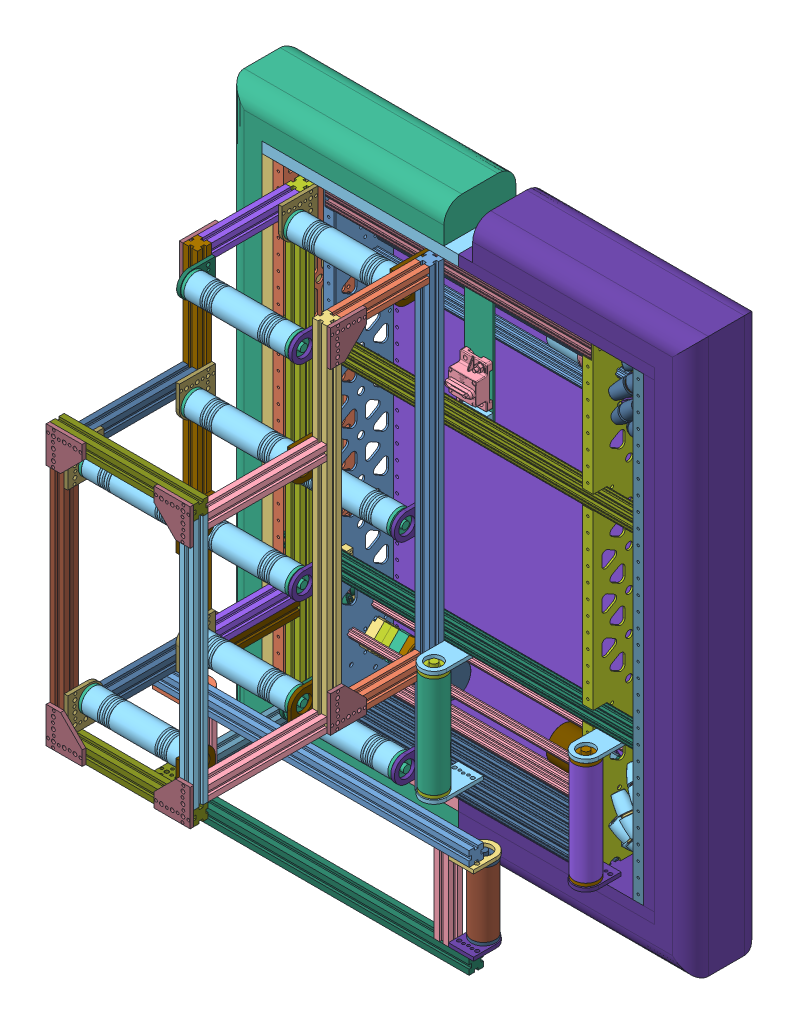
SolidWorks assembly Robot 2020, configuration Default. Lengths in mm. (continued)
Components (placement in the parent): (continued)
- Copy of Fame 2020-1: Copy of Fame 2020 [Default] at origin size (819.15 977.9 171.99) (continued)
  - NEO Gearbox 2-stage Custom v5(Mirror) (2)^Copy of Fame 2020-1: NEO Gearbox 2-stage Custom v5(Mirror) (2)^Copy of Fame 2020 [Default] at (0 0 425) x (1 0 0) z (0 0 -1) size (164.9 90.53 90.53) (virtual) (continued)
    - VersaPlanetary_4_1_Gear_Kit_217-2818 v1(Mirror) (2)^NEO Gearbox 2-stage Custom v5(Mirror) (2)_Copy of Fame 2020-1: VersaPlanetary_4_1_Gear_Kit_217-2818 v1(Mirror) (2)^NEO Gearbox 2-stage Custom v5(Mirror) (2)_Copy of Fame 2020 [Default] at (-15.25 22.225 0) x (0 -0.707107 -0.707107) z (1 0 0) size (35.49 35.49 17.4) (virtual) (continued)
      - 217-2625-010 Rev1(Mirror) (2)^VersaPlanetary_4_1_Gear_Kit_217-2818 v1(Mirror) (2)_NEO Gearbox 2-stage Custom v5(Mirror) (2)_Copy of Fame 2020-4: 217-2625-010 Rev1(Mirror) (2)^VersaPlanetary_4_1_Gear_Kit_217-2818 v1(Mirror) (2)_NEO Gearbox 2-stage Custom v5(Mirror) (2)_Copy of Fame 2020 [Default] at (-45.2382 -508.5855 214.725) x (0.519745 -0.854322 0) z (0 0 1) size (4 4 12) (virtual)
    - 217-2625-026 Rev1(Mirror) (2)^NEO Gearbox 2-stage Custom v5(Mirror) (2)_Copy of Fame 2020-1: 217-2625-026 Rev1(Mirror) (2)^NEO Gearbox 2-stage Custom v5(Mirror) (2)_Copy of Fame 2020 [Default] at (211.875 -317.5 391.6125) x (0 -0.707107 -0.707107) z (1 0 0) size (44.45 42 18.12) (virtual)
    - 217-2742-001 Rev4(Mirror) (2)^NEO Gearbox 2-stage Custom v5(Mirror) (2)_Copy of Fame 2020-1: 217-2742-001 Rev4(Mirror) (2)^NEO Gearbox 2-stage Custom v5(Mirror) (2)_Copy of Fame 2020 [Default] at (218.5752 -317.5 391.6125) x (1 0 0) z (0 -0.63857 0.769564) size (7 28 28) (virtual)
    - 217-2742-001 Rev4(Mirror) (2)^NEO Gearbox 2-stage Custom v5(Mirror) (2)_Copy of Fame 2020-2: 217-2742-001 Rev4(Mirror) (2)^NEO Gearbox 2-stage Custom v5(Mirror) (2)_Copy of Fame 2020 [Default] at (226.5752 -317.5 391.6125) x (1 0 0) z (0 -0.707107 0.707107) size (7 28 28) (virtual)
    - 217-2625-017 Rev1_9714K61(Mirror) (2)^NEO Gearbox 2-stage Custom v5(Mirror) (2)_Copy of Fame 2020-1: 217-2625-017 Rev1_9714K61(Mirror) (2)^NEO Gearbox 2-stage Custom v5(Mirror) (2)_Copy of Fame 2020 [Default] at (225.795 -317.6887 391.9075) x (0 0.983393 -0.181491) z (0 0.181491 0.983393) size (28.51 4.98 27.43) (virtual)
    - 217-2625-025 Rev1(Mirror) (2)^NEO Gearbox 2-stage Custom v5(Mirror) (2)_Copy of Fame 2020-1: 217-2625-025 Rev1(Mirror) (2)^NEO Gearbox 2-stage Custom v5(Mirror) (2)_Copy of Fame 2020 [Default] at (182.475 -317.5 391.6125) x (0 -0.707107 -0.707107) z (1 0 0) size (44.45 42 18) (virtual)
    - 217-2816-001 Rev1(Mirror) (2)^NEO Gearbox 2-stage Custom v5(Mirror) (2)_Copy of Fame 2020-1: 217-2816-001 Rev1(Mirror) (2)^NEO Gearbox 2-stage Custom v5(Mirror) (2)_Copy of Fame 2020 [Default] at (212.025 -317.5 391.6125) x (0 -0.707107 -0.707107) z (-1 0 0) size (42 42 14.5) (virtual)
    - 217-2816-001 Rev1(Mirror) (2)^NEO Gearbox 2-stage Custom v5(Mirror) (2)_Copy of Fame 2020-2: 217-2816-001 Rev1(Mirror) (2)^NEO Gearbox 2-stage Custom v5(Mirror) (2)_Copy of Fame 2020 [Default] at (199.325 -317.5 391.6125) x (0 -0.707107 -0.707107) z (-1 0 0) size (42 42 14.5) (virtual)
    - 217-4649-001 Rev1(Mirror) (2)^NEO Gearbox 2-stage Custom v5(Mirror) (2)_Copy of Fame 2020-1: 217-4649-001 Rev1(Mirror) (2)^NEO Gearbox 2-stage Custom v5(Mirror) (2)_Copy of Fame 2020 [Default] at (185.629 -317.5 391.6125) x (0 -0.707107 -0.707107) z (-1 0 0) size (18 18 13) (virtual)
    - VersaPlanetary_CIM_Adapter_217-4018 v1(Mirror) (2)^NEO Gearbox 2-stage Custom v5(Mirror) (2)_Copy of Fame 2020-1: VersaPlanetary_CIM_Adapter_217-4018 v1(Mirror) (2)^NEO Gearbox 2-stage Custom v5(Mirror) (2)_Copy of Fame 2020 [Default] at (165.15 -317.5 391.6125) x (0 -0.707107 -0.707107) z (0 -0.707107 0.707107) size (64.01 21.55 64.01) (virtual)
    - NEO Motor REV-21-1650 v2(Mirror) (2)^NEO Gearbox 2-stage Custom v5(Mirror) (2)_Copy of Fame 2020-1: NEO Motor REV-21-1650 v2(Mirror) (2)^NEO Gearbox 2-stage Custom v5(Mirror) (2)_Copy of Fame 2020 [Default] at (153.625 -317.5 391.6125) x (0 -0.707107 0.707107) z (-1 0 0) size (61.14 61.02 93.25) (virtual)
    - 3_1 Output Shaft Custom v6(Mirror) (2)^NEO Gearbox 2-stage Custom v5(Mirror) (2)_Copy of Fame 2020-1: 3_1 Output Shaft Custom v6(Mirror) (2)^NEO Gearbox 2-stage Custom v5(Mirror) (2)_Copy of Fame 2020 [Default] at (211.3752 -317.5 391.6125) x (1 0 0) z (0 -0.707107 0.707107) size (48.9 34.7 34.7) (virtual)
  - Left Wheel Assembly v4(Mirror) (2)^Copy of Fame 2020-1: Left Wheel Assembly v4(Mirror) (2)^Copy of Fame 2020 [Default] at (500 0 0) x (1 0 0) z (0 0 -1) size (65.82 166.11 165.01) (virtual)
    - 6_Mecanum_Wheel_Left_217-2799 v1(Mirror) (2)^Left Wheel Assembly v4(Mirror) (2)_Copy of Fame 2020-1: 6_Mecanum_Wheel_Left_217-2799 v1(Mirror) (2)^Left Wheel Assembly v4(Mirror) (2)_Copy of Fame 2020 [Default] x (0 0 -1) z (1 0 0) size (165.01 166.11 65.82) (virtual)
      - 217-2799-001 Rev1(Mirror) (2)^6_Mecanum_Wheel_Left_217-2799 v1(Mirror) (2)_Left Wheel Assembly v4(Mirror) (2)_Copy of Fame 2020-1: 217-2799-001 Rev1(Mirror) (2)^6_Mecanum_Wheel_Left_217-2799 v1(Mirror) (2)_Left Wheel Assembly v4(Mirror) (2)_Copy of Fame 2020 [Default] at (33.3875 -317.5 -234.0098) x (0.707107 0.707107 0) z (0 0 1) size (95.78 100.46 28.55) (virtual)
      - 217-2799-001 Rev1(Mirror) (2)^6_Mecanum_Wheel_Left_217-2799 v1(Mirror) (2)_Left Wheel Assembly v4(Mirror) (2)_Copy of Fame 2020-2: 217-2799-001 Rev1(Mirror) (2)^6_Mecanum_Wheel_Left_217-2799 v1(Mirror) (2)_Left Wheel Assembly v4(Mirror) (2)_Copy of Fame 2020 [Default] at (33.3875 -317.5 -221.3098) x (-0.987688 -0.156434 0) z (0 0 -1) size (95.78 100.46 28.55) (virtual)
      - 217-2799-002 Rev1(Mirror) (2)^6_Mecanum_Wheel_Left_217-2799 v1(Mirror) (2)_Left Wheel Assembly v4(Mirror) (2)_Copy of Fame 2020-1: 217-2799-002 Rev1(Mirror) (2)^6_Mecanum_Wheel_Left_217-2799 v1(Mirror) (2)_Left Wheel Assembly v4(Mirror) (2)_Copy of Fame 2020 [Default] at (4.057 -346.8305 -227.6598) x (-0.707107 0.707107 0) z (0.707107 0.707107 0) size (26.84 25.39 30.1) (virtual)
      - 217-2799-002 Rev1(Mirror) (2)^6_Mecanum_Wheel_Left_217-2799 v1(Mirror) (2)_Left Wheel Assembly v4(Mirror) (2)_Copy of Fame 2020-2: 217-2799-002 Rev1(Mirror) (2)^6_Mecanum_Wheel_Left_217-2799 v1(Mirror) (2)_Left Wheel Assembly v4(Mirror) (2)_Copy of Fame 2020 [Default] at (-7.5815 -323.9888 -227.6598) x (-0.156434 0.987688 0) z (0.987688 0.156434 0) size (26.84 25.39 30.1) (virtual)
      - 217-2799-002 Rev1(Mirror) (2)^6_Mecanum_Wheel_Left_217-2799 v1(Mirror) (2)_Left Wheel Assembly v4(Mirror) (2)_Copy of Fame 2020-3: 217-2799-002 Rev1(Mirror) (2)^6_Mecanum_Wheel_Left_217-2799 v1(Mirror) (2)_Left Wheel Assembly v4(Mirror) (2)_Copy of Fame 2020 [Default] at (-3.5711 -298.6686 -227.6598) x (0.45399 0.891007 0) z (0.891007 -0.45399 0) size (26.84 25.39 30.1) (virtual)
      - 217-2799-002 Rev1(Mirror) (2)^6_Mecanum_Wheel_Left_217-2799 v1(Mirror) (2)_Left Wheel Assembly v4(Mirror) (2)_Copy of Fame 2020-4: 217-2799-002 Rev1(Mirror) (2)^6_Mecanum_Wheel_Left_217-2799 v1(Mirror) (2)_Left Wheel Assembly v4(Mirror) (2)_Copy of Fame 2020 [Default] at (14.5561 -280.5414 -227.6598) x (0.891007 0.45399 0) z (0.45399 -0.891007 0) size (26.84 25.39 30.1) (virtual)
      - 217-2799-002 Rev1(Mirror) (2)^6_Mecanum_Wheel_Left_217-2799 v1(Mirror) (2)_Left Wheel Assembly v4(Mirror) (2)_Copy of Fame 2020-5: 217-2799-002 Rev1(Mirror) (2)^6_Mecanum_Wheel_Left_217-2799 v1(Mirror) (2)_Left Wheel Assembly v4(Mirror) (2)_Copy of Fame 2020 [Default] at (39.8763 -276.531 -227.6598) x (0.987688 -0.156434 0) z (-0.156434 -0.987688 0) size (26.84 25.39 30.1) (virtual)
      - 217-2799-002 Rev1(Mirror) (2)^6_Mecanum_Wheel_Left_217-2799 v1(Mirror) (2)_Left Wheel Assembly v4(Mirror) (2)_Copy of Fame 2020-6: 217-2799-002 Rev1(Mirror) (2)^6_Mecanum_Wheel_Left_217-2799 v1(Mirror) (2)_Left Wheel Assembly v4(Mirror) (2)_Copy of Fame 2020 [Default] at (62.718 -288.1695 -227.6598) x (0.707107 -0.707107 0) z (-0.707107 -0.707107 0) size (26.84 25.39 30.1) (virtual)
      - 217-2799-002 Rev1(Mirror) (2)^6_Mecanum_Wheel_Left_217-2799 v1(Mirror) (2)_Left Wheel Assembly v4(Mirror) (2)_Copy of Fame 2020-7: 217-2799-002 Rev1(Mirror) (2)^6_Mecanum_Wheel_Left_217-2799 v1(Mirror) (2)_Left Wheel Assembly v4(Mirror) (2)_Copy of Fame 2020 [Default] at (74.3565 -311.0112 -227.6598) x (0.156434 -0.987688 0) z (-0.987688 -0.156434 0) size (26.84 25.39 30.1) (virtual)
      - 217-2799-002 Rev1(Mirror) (2)^6_Mecanum_Wheel_Left_217-2799 v1(Mirror) (2)_Left Wheel Assembly v4(Mirror) (2)_Copy of Fame 2020-8: 217-2799-002 Rev1(Mirror) (2)^6_Mecanum_Wheel_Left_217-2799 v1(Mirror) (2)_Left Wheel Assembly v4(Mirror) (2)_Copy of Fame 2020 [Default] at (70.3461 -336.3314 -227.6598) x (-0.45399 -0.891007 0) z (-0.891007 0.45399 0) size (26.84 25.39 30.1) (virtual)
      - 217-2799-002 Rev1(Mirror) (2)^6_Mecanum_Wheel_Left_217-2799 v1(Mirror) (2)_Left Wheel Assembly v4(Mirror) (2)_Copy of Fame 2020-9: 217-2799-002 Rev1(Mirror) (2)^6_Mecanum_Wheel_Left_217-2799 v1(Mirror) (2)_Left Wheel Assembly v4(Mirror) (2)_Copy of Fame 2020 [Default] at (52.2189 -354.4586 -227.6598) x (-0.891007 -0.45399 0) z (-0.45399 0.891007 0) size (26.84 25.39 30.1) (virtual)
      - 217-2799-002 Rev1(Mirror) (2)^6_Mecanum_Wheel_Left_217-2799 v1(Mirror) (2)_Left Wheel Assembly v4(Mirror) (2)_Copy of Fame 2020-10: 217-2799-002 Rev1(Mirror) (2)^6_Mecanum_Wheel_Left_217-2799 v1(Mirror) (2)_Left Wheel Assembly v4(Mirror) (2)_Copy of Fame 2020 [Default] at (26.8987 -358.469 -227.6598) x (-0.987688 0.156434 0) z (0.156434 0.987688 0) size (26.84 25.39 30.1) (virtual)
      - 217-2586-003 Rev2(Mirror) (2)^6_Mecanum_Wheel_Left_217-2799 v1(Mirror) (2)_Left Wheel Assembly v4(Mirror) (2)_Copy of Fame 2020-1: 217-2586-003 Rev2(Mirror) (2)^6_Mecanum_Wheel_Left_217-2799 v1(Mirror) (2)_Left Wheel Assembly v4(Mirror) (2)_Copy of Fame 2020 [Default] at (-13.4676 -358.6894 -223.6536) x (0.41944 0.854155 -0.30739) z (0.757674 -0.142894 0.636798) size (19.46 28.57 19.46) (virtual)
      - 217-2586-003 Rev2(Mirror) (2)^6_Mecanum_Wheel_Left_217-2799 v1(Mirror) (2)_Left Wheel Assembly v4(Mirror) (2)_Copy of Fame 2020-2: 217-2586-003 Rev2(Mirror) (2)^6_Mecanum_Wheel_Left_217-2799 v1(Mirror) (2)_Left Wheel Assembly v4(Mirror) (2)_Copy of Fame 2020 [Default] at (-7.8019 -364.3551 -231.666) x (0.847342 0.451134 0.280161) z (-0.17892 0.739241 -0.649238) size (19.46 28.57 19.46) (virtual)
      - 217-2586-003 Rev2(Mirror) (2)^6_Mecanum_Wheel_Left_217-2799 v1(Mirror) (2)_Left Wheel Assembly v4(Mirror) (2)_Copy of Fame 2020-3: 217-2586-003 Rev2(Mirror) (2)^6_Mecanum_Wheel_Left_217-2799 v1(Mirror) (2)_Left Wheel Assembly v4(Mirror) (2)_Copy of Fame 2020 [Default] at (-27.4761 -331.196 -231.666) x (0.950684 -0.13308 0.280161) z (0.289766 0.703225 -0.649238) size (19.46 28.57 19.46) (virtual)
      - 217-2586-003 Rev2(Mirror) (2)^6_Mecanum_Wheel_Left_217-2799 v1(Mirror) (2)_Left Wheel Assembly v4(Mirror) (2)_Copy of Fame 2020-4: 217-2586-003 Rev2(Mirror) (2)^6_Mecanum_Wheel_Left_217-2799 v1(Mirror) (2)_Left Wheel Assembly v4(Mirror) (2)_Copy of Fame 2020 [Default] at (-23.9025 -292.8056 -231.666) x (0.690897 -0.666462 0.280161) z (0.647771 0.398601 -0.649238) size (19.46 28.57 19.46) (virtual)
      - 217-2586-003 Rev2(Mirror) (2)^6_Mecanum_Wheel_Left_217-2799 v1(Mirror) (2)_Left Wheel Assembly v4(Mirror) (2)_Copy of Fame 2020-5: 217-2586-003 Rev2(Mirror) (2)^6_Mecanum_Wheel_Left_217-2799 v1(Mirror) (2)_Left Wheel Assembly v4(Mirror) (2)_Copy of Fame 2020 [Default] at (1.5539 -263.8475 -231.666) x (0.167211 -0.945278 0.280161) z (0.75835 -0.058276 -0.649238) size (19.46 28.57 19.46) (virtual)
      - 217-2586-003 Rev2(Mirror) (2)^6_Mecanum_Wheel_Left_217-2799 v1(Mirror) (2)_Left Wheel Assembly v4(Mirror) (2)_Copy of Fame 2020-6: 217-2586-003 Rev2(Mirror) (2)^6_Mecanum_Wheel_Left_217-2799 v1(Mirror) (2)_Left Wheel Assembly v4(Mirror) (2)_Copy of Fame 2020 [Default] at (39.1697 -255.3829 -231.666) x (-0.420344 -0.86303 0.280161) z (0.579264 -0.492893 -0.649238) size (19.46 28.57 19.46) (virtual)
      - 217-2586-003 Rev2(Mirror) (2)^6_Mecanum_Wheel_Left_217-2799 v1(Mirror) (2)_Left Wheel Assembly v4(Mirror) (2)_Copy of Fame 2020-7: 217-2586-003 Rev2(Mirror) (2)^6_Mecanum_Wheel_Left_217-2799 v1(Mirror) (2)_Left Wheel Assembly v4(Mirror) (2)_Copy of Fame 2020 [Default] at (74.5769 -270.6449 -231.666) x (-0.847342 -0.451134 0.280161) z (0.17892 -0.739241 -0.649238) size (19.46 28.57 19.46) (virtual)
      - 217-2586-003 Rev2(Mirror) (2)^6_Mecanum_Wheel_Left_217-2799 v1(Mirror) (2)_Left Wheel Assembly v4(Mirror) (2)_Copy of Fame 2020-8: 217-2586-003 Rev2(Mirror) (2)^6_Mecanum_Wheel_Left_217-2799 v1(Mirror) (2)_Left Wheel Assembly v4(Mirror) (2)_Copy of Fame 2020 [Default] at (94.2511 -303.804 -231.666) x (-0.950684 0.13308 0.280161) z (-0.289766 -0.703225 -0.649238) size (19.46 28.57 19.46) (virtual)
      - 217-2586-003 Rev2(Mirror) (2)^6_Mecanum_Wheel_Left_217-2799 v1(Mirror) (2)_Left Wheel Assembly v4(Mirror) (2)_Copy of Fame 2020-9: 217-2586-003 Rev2(Mirror) (2)^6_Mecanum_Wheel_Left_217-2799 v1(Mirror) (2)_Left Wheel Assembly v4(Mirror) (2)_Copy of Fame 2020 [Default] at (90.6775 -342.1944 -231.666) x (-0.690897 0.666462 0.280161) z (-0.647771 -0.398601 -0.649238) size (19.46 28.57 19.46) (virtual)
      - 217-2586-003 Rev2(Mirror) (2)^6_Mecanum_Wheel_Left_217-2799 v1(Mirror) (2)_Left Wheel Assembly v4(Mirror) (2)_Copy of Fame 2020-10: 217-2586-003 Rev2(Mirror) (2)^6_Mecanum_Wheel_Left_217-2799 v1(Mirror) (2)_Left Wheel Assembly v4(Mirror) (2)_Copy of Fame 2020 [Default] at (65.2211 -371.1525 -231.666) x (-0.167211 0.945278 0.280161) z (-0.75835 0.058276 -0.649238) size (19.46 28.57 19.46) (virtual)
      - 217-2586-003 Rev2(Mirror) (2)^6_Mecanum_Wheel_Left_217-2799 v1(Mirror) (2)_Left Wheel Assembly v4(Mirror) (2)_Copy of Fame 2020-11: 217-2586-003 Rev2(Mirror) (2)^6_Mecanum_Wheel_Left_217-2799 v1(Mirror) (2)_Left Wheel Assembly v4(Mirror) (2)_Copy of Fame 2020 [Default] at (27.6053 -379.6171 -231.666) x (0.420344 0.86303 0.280161) z (-0.579264 0.492893 -0.649238) size (19.46 28.57 19.46) (virtual)
      - 217-2586-003 Rev2(Mirror) (2)^6_Mecanum_Wheel_Left_217-2799 v1(Mirror) (2)_Left Wheel Assembly v4(Mirror) (2)_Copy of Fame 2020-12: 217-2586-003 Rev2(Mirror) (2)^6_Mecanum_Wheel_Left_217-2799 v1(Mirror) (2)_Left Wheel Assembly v4(Mirror) (2)_Copy of Fame 2020 [Default] at (-28.7296 -323.2822 -223.6536) x (0.841394 0.444485 -0.30739) z (0.52898 -0.560953 0.636798) size (19.46 28.57 19.46) (virtual)
      - 217-2586-003 Rev2(Mirror) (2)^6_Mecanum_Wheel_Left_217-2799 v1(Mirror) (2)_Left Wheel Assembly v4(Mirror) (2)_Copy of Fame 2020-13: 217-2586-003 Rev2(Mirror) (2)^6_Mecanum_Wheel_Left_217-2799 v1(Mirror) (2)_Left Wheel Assembly v4(Mirror) (2)_Copy of Fame 2020 [Default] at (-20.265 -285.6664 -223.6536) x (0.941964 -0.134963 -0.30739) z (0.098234 -0.764747 0.636798) size (19.46 28.57 19.46) (virtual)
      - 217-2586-003 Rev2(Mirror) (2)^6_Mecanum_Wheel_Left_217-2799 v1(Mirror) (2)_Left Wheel Assembly v4(Mirror) (2)_Copy of Fame 2020-14: 217-2586-003 Rev2(Mirror) (2)^6_Mecanum_Wheel_Left_217-2799 v1(Mirror) (2)_Left Wheel Assembly v4(Mirror) (2)_Copy of Fame 2020 [Default] at (8.6931 -260.21 -223.6536) x (0.682736 -0.66286 -0.30739) z (-0.370035 -0.676434 0.636798) size (19.46 28.57 19.46) (virtual)
      - 217-2586-003 Rev2(Mirror) (2)^6_Mecanum_Wheel_Left_217-2799 v1(Mirror) (2)_Left Wheel Assembly v4(Mirror) (2)_Copy of Fame 2020-15: 217-2586-003 Rev2(Mirror) (2)^6_Mecanum_Wheel_Left_217-2799 v1(Mirror) (2)_Left Wheel Assembly v4(Mirror) (2)_Copy of Fame 2020 [Default] at (47.0835 -256.6364 -223.6536) x (0.162726 -0.937567 -0.30739) z (-0.696962 -0.329746 0.636798) size (19.46 28.57 19.46) (virtual)
      - 217-2586-003 Rev2(Mirror) (2)^6_Mecanum_Wheel_Left_217-2799 v1(Mirror) (2)_Left Wheel Assembly v4(Mirror) (2)_Copy of Fame 2020-16: 217-2586-003 Rev2(Mirror) (2)^6_Mecanum_Wheel_Left_217-2799 v1(Mirror) (2)_Left Wheel Assembly v4(Mirror) (2)_Copy of Fame 2020 [Default] at (80.2426 -276.3106 -223.6536) x (-0.41944 -0.854155 -0.30739) z (-0.757674 0.142894 0.636798) size (19.46 28.57 19.46) (virtual)
      - 217-2586-003 Rev2(Mirror) (2)^6_Mecanum_Wheel_Left_217-2799 v1(Mirror) (2)_Left Wheel Assembly v4(Mirror) (2)_Copy of Fame 2020-17: 217-2586-003 Rev2(Mirror) (2)^6_Mecanum_Wheel_Left_217-2799 v1(Mirror) (2)_Left Wheel Assembly v4(Mirror) (2)_Copy of Fame 2020 [Default] at (95.5046 -311.7178 -223.6536) x (-0.841394 -0.444485 -0.30739) z (-0.52898 0.560953 0.636798) size (19.46 28.57 19.46) (virtual)
      - 217-2586-003 Rev2(Mirror) (2)^6_Mecanum_Wheel_Left_217-2799 v1(Mirror) (2)_Left Wheel Assembly v4(Mirror) (2)_Copy of Fame 2020-18: 217-2586-003 Rev2(Mirror) (2)^6_Mecanum_Wheel_Left_217-2799 v1(Mirror) (2)_Left Wheel Assembly v4(Mirror) (2)_Copy of Fame 2020 [Default] at (87.04 -349.3336 -223.6536) x (-0.941964 0.134963 -0.30739) z (-0.098234 0.764747 0.636798) size (19.46 28.57 19.46) (virtual)
      - 217-2586-003 Rev2(Mirror) (2)^6_Mecanum_Wheel_Left_217-2799 v1(Mirror) (2)_Left Wheel Assembly v4(Mirror) (2)_Copy of Fame 2020-19: 217-2586-003 Rev2(Mirror) (2)^6_Mecanum_Wheel_Left_217-2799 v1(Mirror) (2)_Left Wheel Assembly v4(Mirror) (2)_Copy of Fame 2020 [Default] at (58.0819 -374.79 -223.6536) x (-0.682736 0.66286 -0.30739) z (0.370035 0.676434 0.636798) size (19.46 28.57 19.46) (virtual)
      - 217-2586-003 Rev2(Mirror) (2)^6_Mecanum_Wheel_Left_217-2799 v1(Mirror) (2)_Left Wheel Assembly v4(Mirror) (2)_Copy of Fame 2020-20: 217-2586-003 Rev2(Mirror) (2)^6_Mecanum_Wheel_Left_217-2799 v1(Mirror) (2)_Left Wheel Assembly v4(Mirror) (2)_Copy of Fame 2020 [Default] at (19.6915 -378.3636 -223.6536) x (-0.162726 0.937567 -0.30739) z (0.696962 0.329746 0.636798) size (19.46 28.57 19.46) (virtual)
      - 217-2586-004 Rev1(Mirror) (2)^6_Mecanum_Wheel_Left_217-2799 v1(Mirror) (2)_Left Wheel Assembly v4(Mirror) (2)_Copy of Fame 2020-1: 217-2586-004 Rev1(Mirror) (2)^6_Mecanum_Wheel_Left_217-2799 v1(Mirror) (2)_Left Wheel Assembly v4(Mirror) (2)_Copy of Fame 2020 [Default] at (-10.3479 -361.809 -228.0654) x (-0.690521 -0.722949 0.02293) z (-0.522667 0.476807 -0.706735) size (25.9 28.58 25.9) (virtual)
      - 217-2586-004 Rev1(Mirror) (2)^6_Mecanum_Wheel_Left_217-2799 v1(Mirror) (2)_Left Wheel Assembly v4(Mirror) (2)_Copy of Fame 2020-2: 217-2586-004 Rev1(Mirror) (2)^6_Mecanum_Wheel_Left_217-2799 v1(Mirror) (2)_Left Wheel Assembly v4(Mirror) (2)_Copy of Fame 2020 [Default] at (-10.9209 -361.2361 -227.2551) x (0.01458 -0.811521 0.584142) z (0.865903 0.302381 0.39847) size (25.9 28.58 25.9) (virtual)
      - 217-2586-004 Rev1(Mirror) (2)^6_Mecanum_Wheel_Left_217-2799 v1(Mirror) (2)_Left Wheel Assembly v4(Mirror) (2)_Copy of Fame 2020-3: 217-2586-004 Rev1(Mirror) (2)^6_Mecanum_Wheel_Left_217-2799 v1(Mirror) (2)_Left Wheel Assembly v4(Mirror) (2)_Copy of Fame 2020 [Default] at (-28.1662 -326.8394 -227.2551) x (-0.465204 -0.665104 0.584142) z (0.878265 -0.264334 0.39847) size (25.9 28.58 25.9) (virtual)
      - 217-2586-004 Rev1(Mirror) (2)^6_Mecanum_Wheel_Left_217-2799 v1(Mirror) (2)_Left Wheel Assembly v4(Mirror) (2)_Copy of Fame 2020-4: 217-2586-004 Rev1(Mirror) (2)^6_Mecanum_Wheel_Left_217-2799 v1(Mirror) (2)_Left Wheel Assembly v4(Mirror) (2)_Copy of Fame 2020 [Default] at (-21.9 -288.8754 -227.2551) x (-0.767297 -0.26464 0.584142) z (0.55516 -0.730082 0.39847) size (25.9 28.58 25.9) (virtual)
      - 217-2586-004 Rev1(Mirror) (2)^6_Mecanum_Wheel_Left_217-2799 v1(Mirror) (2)_Left Wheel Assembly v4(Mirror) (2)_Copy of Fame 2020-5: 217-2586-004 Rev1(Mirror) (2)^6_Mecanum_Wheel_Left_217-2799 v1(Mirror) (2)_Left Wheel Assembly v4(Mirror) (2)_Copy of Fame 2020 [Default] at (5.484 -261.845 -227.2551) x (-0.776308 0.236907 0.584142) z (0.020002 -0.916963 0.39847) size (25.9 28.58 25.9) (virtual)
      - 217-2586-004 Rev1(Mirror) (2)^6_Mecanum_Wheel_Left_217-2799 v1(Mirror) (2)_Left Wheel Assembly v4(Mirror) (2)_Copy of Fame 2020-6: 217-2586-004 Rev1(Mirror) (2)^6_Mecanum_Wheel_Left_217-2799 v1(Mirror) (2)_Left Wheel Assembly v4(Mirror) (2)_Copy of Fame 2020 [Default] at (43.5263 -256.0729 -227.2551) x (-0.488796 0.647964 0.584142) z (-0.522795 -0.753596 0.39847) size (25.9 28.58 25.9) (virtual)
      - 217-2586-004 Rev1(Mirror) (2)^6_Mecanum_Wheel_Left_217-2799 v1(Mirror) (2)_Left Wheel Assembly v4(Mirror) (2)_Copy of Fame 2020-7: 217-2586-004 Rev1(Mirror) (2)^6_Mecanum_Wheel_Left_217-2799 v1(Mirror) (2)_Left Wheel Assembly v4(Mirror) (2)_Copy of Fame 2020 [Default] at (77.6959 -273.7639 -227.2551) x (-0.01458 0.811521 0.584142) z (-0.865903 -0.302381 0.39847) size (25.9 28.58 25.9) (virtual)
      - 217-2586-004 Rev1(Mirror) (2)^6_Mecanum_Wheel_Left_217-2799 v1(Mirror) (2)_Left Wheel Assembly v4(Mirror) (2)_Copy of Fame 2020-8: 217-2586-004 Rev1(Mirror) (2)^6_Mecanum_Wheel_Left_217-2799 v1(Mirror) (2)_Left Wheel Assembly v4(Mirror) (2)_Copy of Fame 2020 [Default] at (94.9412 -308.1606 -227.2551) x (0.465204 0.665104 0.584142) z (-0.878265 0.264334 0.39847) size (25.9 28.58 25.9) (virtual)
      - 217-2586-004 Rev1(Mirror) (2)^6_Mecanum_Wheel_Left_217-2799 v1(Mirror) (2)_Left Wheel Assembly v4(Mirror) (2)_Copy of Fame 2020-9: 217-2586-004 Rev1(Mirror) (2)^6_Mecanum_Wheel_Left_217-2799 v1(Mirror) (2)_Left Wheel Assembly v4(Mirror) (2)_Copy of Fame 2020 [Default] at (88.675 -346.1246 -227.2551) x (0.767297 0.26464 0.584142) z (-0.55516 0.730082 0.39847) size (25.9 28.58 25.9) (virtual)
      - 217-2586-004 Rev1(Mirror) (2)^6_Mecanum_Wheel_Left_217-2799 v1(Mirror) (2)_Left Wheel Assembly v4(Mirror) (2)_Copy of Fame 2020-10: 217-2586-004 Rev1(Mirror) (2)^6_Mecanum_Wheel_Left_217-2799 v1(Mirror) (2)_Left Wheel Assembly v4(Mirror) (2)_Copy of Fame 2020 [Default] at (61.291 -373.155 -227.2551) x (0.776308 -0.236907 0.584142) z (-0.020002 0.916963 0.39847) size (25.9 28.58 25.9) (virtual)
      - 217-2586-004 Rev1(Mirror) (2)^6_Mecanum_Wheel_Left_217-2799 v1(Mirror) (2)_Left Wheel Assembly v4(Mirror) (2)_Copy of Fame 2020-11: 217-2586-004 Rev1(Mirror) (2)^6_Mecanum_Wheel_Left_217-2799 v1(Mirror) (2)_Left Wheel Assembly v4(Mirror) (2)_Copy of Fame 2020 [Default] at (23.2487 -378.9271 -227.2551) x (0.488796 -0.647964 0.584142) z (0.522795 0.753596 0.39847) size (25.9 28.58 25.9) (virtual)
      - 217-2586-004 Rev1(Mirror) (2)^6_Mecanum_Wheel_Left_217-2799 v1(Mirror) (2)_Left Wheel Assembly v4(Mirror) (2)_Copy of Fame 2020-12: 217-2586-004 Rev1(Mirror) (2)^6_Mecanum_Wheel_Left_217-2799 v1(Mirror) (2)_Left Wheel Assembly v4(Mirror) (2)_Copy of Fame 2020 [Default] at (-28.0394 -327.6397 -228.0654) x (-0.983582 -0.179 0.02293) z (-0.142587 0.692961 -0.706735) size (25.9 28.58 25.9) (virtual)
      - 217-2586-004 Rev1(Mirror) (2)^6_Mecanum_Wheel_Left_217-2799 v1(Mirror) (2)_Left Wheel Assembly v4(Mirror) (2)_Copy of Fame 2020-13: 217-2586-004 Rev1(Mirror) (2)^6_Mecanum_Wheel_Left_217-2799 v1(Mirror) (2)_Left Wheel Assembly v4(Mirror) (2)_Copy of Fame 2020 [Default] at (-22.2679 -289.5974 -228.0654) x (-0.900948 0.433321 0.02293) z (0.291957 0.644427 -0.706735) size (25.9 28.58 25.9) (virtual)
      - 217-2586-004 Rev1(Mirror) (2)^6_Mecanum_Wheel_Left_217-2799 v1(Mirror) (2)_Left Wheel Assembly v4(Mirror) (2)_Copy of Fame 2020-14: 217-2586-004 Rev1(Mirror) (2)^6_Mecanum_Wheel_Left_217-2799 v1(Mirror) (2)_Left Wheel Assembly v4(Mirror) (2)_Copy of Fame 2020 [Default] at (4.7621 -262.2129 -228.0654) x (-0.474183 0.880128 0.02293) z (0.614983 0.349745 -0.706735) size (25.9 28.58 25.9) (virtual)
      - 217-2586-004 Rev1(Mirror) (2)^6_Mecanum_Wheel_Left_217-2799 v1(Mirror) (2)_Left Wheel Assembly v4(Mirror) (2)_Copy of Fame 2020-15: 217-2586-004 Rev1(Mirror) (2)^6_Mecanum_Wheel_Left_217-2799 v1(Mirror) (2)_Left Wheel Assembly v4(Mirror) (2)_Copy of Fame 2020 [Default] at (42.726 -255.9462 -228.0654) x (0.133704 0.990756 0.02293) z (0.703107 -0.078529 -0.706735) size (25.9 28.58 25.9) (virtual)
      - 217-2586-004 Rev1(Mirror) (2)^6_Mecanum_Wheel_Left_217-2799 v1(Mirror) (2)_Left Wheel Assembly v4(Mirror) (2)_Copy of Fame 2020-16: 217-2586-004 Rev1(Mirror) (2)^6_Mecanum_Wheel_Left_217-2799 v1(Mirror) (2)_Left Wheel Assembly v4(Mirror) (2)_Copy of Fame 2020 [Default] at (77.1229 -273.191 -228.0654) x (0.690521 0.722949 0.02293) z (0.522667 -0.476807 -0.706735) size (25.9 28.58 25.9) (virtual)
      - 217-2586-004 Rev1(Mirror) (2)^6_Mecanum_Wheel_Left_217-2799 v1(Mirror) (2)_Left Wheel Assembly v4(Mirror) (2)_Copy of Fame 2020-17: 217-2586-004 Rev1(Mirror) (2)^6_Mecanum_Wheel_Left_217-2799 v1(Mirror) (2)_Left Wheel Assembly v4(Mirror) (2)_Copy of Fame 2020 [Default] at (94.8144 -307.3603 -228.0654) x (0.983582 0.179 0.02293) z (0.142587 -0.692961 -0.706735) size (25.9 28.58 25.9) (virtual)
      - 217-2586-004 Rev1(Mirror) (2)^6_Mecanum_Wheel_Left_217-2799 v1(Mirror) (2)_Left Wheel Assembly v4(Mirror) (2)_Copy of Fame 2020-18: 217-2586-004 Rev1(Mirror) (2)^6_Mecanum_Wheel_Left_217-2799 v1(Mirror) (2)_Left Wheel Assembly v4(Mirror) (2)_Copy of Fame 2020 [Default] at (89.0429 -345.4026 -228.0654) x (0.900948 -0.433321 0.02293) z (-0.291957 -0.644427 -0.706735) size (25.9 28.58 25.9) (virtual)
      - 217-2586-004 Rev1(Mirror) (2)^6_Mecanum_Wheel_Left_217-2799 v1(Mirror) (2)_Left Wheel Assembly v4(Mirror) (2)_Copy of Fame 2020-19: 217-2586-004 Rev1(Mirror) (2)^6_Mecanum_Wheel_Left_217-2799 v1(Mirror) (2)_Left Wheel Assembly v4(Mirror) (2)_Copy of Fame 2020 [Default] at (62.0129 -372.7871 -228.0654) x (0.474183 -0.880128 0.02293) z (-0.614983 -0.349745 -0.706735) size (25.9 28.58 25.9) (virtual)
      - 217-2586-004 Rev1(Mirror) (2)^6_Mecanum_Wheel_Left_217-2799 v1(Mirror) (2)_Left Wheel Assembly v4(Mirror) (2)_Copy of Fame 2020-20: 217-2586-004 Rev1(Mirror) (2)^6_Mecanum_Wheel_Left_217-2799 v1(Mirror) (2)_Left Wheel Assembly v4(Mirror) (2)_Copy of Fame 2020 [Default] at (24.049 -379.0538 -228.0654) x (-0.133704 -0.990756 0.02293) z (-0.703107 0.078529 -0.706735) size (25.9 28.58 25.9) (virtual)
      - 217-2586-007 Rev1(Mirror) (2)^6_Mecanum_Wheel_Left_217-2799 v1(Mirror) (2)_Left Wheel Assembly v4(Mirror) (2)_Copy of Fame 2020-1: 217-2586-007 Rev1(Mirror) (2)^6_Mecanum_Wheel_Left_217-2799 v1(Mirror) (2)_Left Wheel Assembly v4(Mirror) (2)_Copy of Fame 2020 [Default] at (-10.6347 -361.5222 -227.6598) x (0.5 -0.5 -0.707107) z (0.709055 0.705148 0.002763) size (61.72 5 5) (virtual)
      - 217-2586-007 Rev1(Mirror) (2)^6_Mecanum_Wheel_Left_217-2799 v1(Mirror) (2)_Left Wheel Assembly v4(Mirror) (2)_Copy of Fame 2020-2: 217-2586-007 Rev1(Mirror) (2)^6_Mecanum_Wheel_Left_217-2799 v1(Mirror) (2)_Left Wheel Assembly v4(Mirror) (2)_Copy of Fame 2020 [Default] at (-28.1029 -327.2391 -227.6598) x (0.110616 -0.698401 -0.707107) z (0.988113 0.153705 0.002763) size (61.72 5 5) (virtual)
      - 217-2586-007 Rev1(Mirror) (2)^6_Mecanum_Wheel_Left_217-2799 v1(Mirror) (2)_Left Wheel Assembly v4(Mirror) (2)_Copy of Fame 2020-3: 217-2586-007 Rev1(Mirror) (2)^6_Mecanum_Wheel_Left_217-2799 v1(Mirror) (2)_Left Wheel Assembly v4(Mirror) (2)_Copy of Fame 2020 [Default] at (-22.0838 -289.236 -227.6598) x (-0.32102 -0.630037 -0.707107) z (0.889746 -0.456448 0.002763) size (61.72 5 5) (virtual)
      - 217-2586-007 Rev1(Mirror) (2)^6_Mecanum_Wheel_Left_217-2799 v1(Mirror) (2)_Left Wheel Assembly v4(Mirror) (2)_Copy of Fame 2020-4: 217-2586-007 Rev1(Mirror) (2)^6_Mecanum_Wheel_Left_217-2799 v1(Mirror) (2)_Left Wheel Assembly v4(Mirror) (2)_Copy of Fame 2020 [Default] at (5.1235 -262.0287 -227.6598) x (-0.630037 -0.32102 -0.707107) z (0.451526 -0.892254 0.002763) size (61.72 5 5) (virtual)
      - 217-2586-007 Rev1(Mirror) (2)^6_Mecanum_Wheel_Left_217-2799 v1(Mirror) (2)_Left Wheel Assembly v4(Mirror) (2)_Copy of Fame 2020-5: 217-2586-007 Rev1(Mirror) (2)^6_Mecanum_Wheel_Left_217-2799 v1(Mirror) (2)_Left Wheel Assembly v4(Mirror) (2)_Copy of Fame 2020 [Default] at (43.1266 -256.0096 -227.6598) x (-0.698401 0.110616 -0.707107) z (-0.159162 -0.987249 0.002763) size (61.72 5 5) (virtual)
      - 217-2586-007 Rev1(Mirror) (2)^6_Mecanum_Wheel_Left_217-2799 v1(Mirror) (2)_Left Wheel Assembly v4(Mirror) (2)_Copy of Fame 2020-6: 217-2586-007 Rev1(Mirror) (2)^6_Mecanum_Wheel_Left_217-2799 v1(Mirror) (2)_Left Wheel Assembly v4(Mirror) (2)_Copy of Fame 2020 [Default] at (77.4097 -273.4778 -227.6598) x (-0.5 0.5 -0.707107) z (-0.709055 -0.705148 0.002763) size (61.72 5 5) (virtual)
      - 217-2586-007 Rev1(Mirror) (2)^6_Mecanum_Wheel_Left_217-2799 v1(Mirror) (2)_Left Wheel Assembly v4(Mirror) (2)_Copy of Fame 2020-7: 217-2586-007 Rev1(Mirror) (2)^6_Mecanum_Wheel_Left_217-2799 v1(Mirror) (2)_Left Wheel Assembly v4(Mirror) (2)_Copy of Fame 2020 [Default] at (94.8779 -307.7609 -227.6598) x (-0.110616 0.698401 -0.707107) z (-0.988113 -0.153705 0.002763) size (61.72 5 5) (virtual)
      - 217-2586-007 Rev1(Mirror) (2)^6_Mecanum_Wheel_Left_217-2799 v1(Mirror) (2)_Left Wheel Assembly v4(Mirror) (2)_Copy of Fame 2020-8: 217-2586-007 Rev1(Mirror) (2)^6_Mecanum_Wheel_Left_217-2799 v1(Mirror) (2)_Left Wheel Assembly v4(Mirror) (2)_Copy of Fame 2020 [Default] at (88.8588 -345.764 -227.6598) x (0.32102 0.630037 -0.707107) z (-0.889746 0.456448 0.002763) size (61.72 5 5) (virtual)
      - 217-2586-007 Rev1(Mirror) (2)^6_Mecanum_Wheel_Left_217-2799 v1(Mirror) (2)_Left Wheel Assembly v4(Mirror) (2)_Copy of Fame 2020-9: 217-2586-007 Rev1(Mirror) (2)^6_Mecanum_Wheel_Left_217-2799 v1(Mirror) (2)_Left Wheel Assembly v4(Mirror) (2)_Copy of Fame 2020 [Default] at (61.6515 -372.9713 -227.6598) x (0.630037 0.32102 -0.707107) z (-0.451526 0.892254 0.002763) size (61.72 5 5) (virtual)
      - 217-2586-007 Rev1(Mirror) (2)^6_Mecanum_Wheel_Left_217-2799 v1(Mirror) (2)_Left Wheel Assembly v4(Mirror) (2)_Copy of Fame 2020-10: 217-2586-007 Rev1(Mirror) (2)^6_Mecanum_Wheel_Left_217-2799 v1(Mirror) (2)_Left Wheel Assembly v4(Mirror) (2)_Copy of Fame 2020 [Default] at (23.6484 -378.9904 -227.6598) x (0.698401 -0.110616 -0.707107) z (0.159162 0.987249 0.002763) size (61.72 5 5) (virtual)
      - 217-2586-008 Rev1(Mirror) (2)^6_Mecanum_Wheel_Left_217-2799 v1(Mirror) (2)_Left Wheel Assembly v4(Mirror) (2)_Copy of Fame 2020-1: 217-2586-008 Rev1(Mirror) (2)^6_Mecanum_Wheel_Left_217-2799 v1(Mirror) (2)_Left Wheel Assembly v4(Mirror) (2)_Copy of Fame 2020 [Default] at (53.3583 -330.4692 -227.5328) x (0.544639 0.838671 0) z (0 0 -1) size (7.33 6.35 31.75) (virtual)
      - 217-2586-008 Rev1(Mirror) (2)^6_Mecanum_Wheel_Left_217-2799 v1(Mirror) (2)_Left Wheel Assembly v4(Mirror) (2)_Copy of Fame 2020-2: 217-2586-008 Rev1(Mirror) (2)^6_Mecanum_Wheel_Left_217-2799 v1(Mirror) (2)_Left Wheel Assembly v4(Mirror) (2)_Copy of Fame 2020 [Default] at (32.1413 -341.2799 -227.5328) x (0.99863 -0.052336 0) z (0 0 -1) size (7.33 6.35 31.75) (virtual)
      - 217-2586-008 Rev1(Mirror) (2)^6_Mecanum_Wheel_Left_217-2799 v1(Mirror) (2)_Left Wheel Assembly v4(Mirror) (2)_Copy of Fame 2020-3: 217-2586-008 Rev1(Mirror) (2)^6_Mecanum_Wheel_Left_217-2799 v1(Mirror) (2)_Left Wheel Assembly v4(Mirror) (2)_Copy of Fame 2020 [Default] at (12.1704 -328.3106 -227.5328) x (0.45399 -0.891007 0) z (0 0 -1) size (7.33 6.35 31.75) (virtual)
      - 217-2586-008 Rev1(Mirror) (2)^6_Mecanum_Wheel_Left_217-2799 v1(Mirror) (2)_Left Wheel Assembly v4(Mirror) (2)_Copy of Fame 2020-4: 217-2586-008 Rev1(Mirror) (2)^6_Mecanum_Wheel_Left_217-2799 v1(Mirror) (2)_Left Wheel Assembly v4(Mirror) (2)_Copy of Fame 2020 [Default] at (13.4167 -304.5308 -227.5328) x (-0.544639 -0.838671 0) z (0 0 -1) size (7.33 6.35 31.75) (virtual)
      - 217-2586-008 Rev1(Mirror) (2)^6_Mecanum_Wheel_Left_217-2799 v1(Mirror) (2)_Left Wheel Assembly v4(Mirror) (2)_Copy of Fame 2020-5: 217-2586-008 Rev1(Mirror) (2)^6_Mecanum_Wheel_Left_217-2799 v1(Mirror) (2)_Left Wheel Assembly v4(Mirror) (2)_Copy of Fame 2020 [Default] at (34.6337 -293.7201 -227.5328) x (-0.99863 0.052336 0) z (0 0 -1) size (7.33 6.35 31.75) (virtual)
      - 217-2586-008 Rev1(Mirror) (2)^6_Mecanum_Wheel_Left_217-2799 v1(Mirror) (2)_Left Wheel Assembly v4(Mirror) (2)_Copy of Fame 2020-6: 217-2586-008 Rev1(Mirror) (2)^6_Mecanum_Wheel_Left_217-2799 v1(Mirror) (2)_Left Wheel Assembly v4(Mirror) (2)_Copy of Fame 2020 [Default] at (54.6046 -306.6894 -227.5328) x (-0.45399 0.891007 0) z (0 0 -1) size (7.33 6.35 31.75) (virtual)
      - NUT-832-NYLOCK(Mirror) (2)^6_Mecanum_Wheel_Left_217-2799 v1(Mirror) (2)_Left Wheel Assembly v4(Mirror) (2)_Copy of Fame 2020-1: NUT-832-NYLOCK(Mirror) (2)^6_Mecanum_Wheel_Left_217-2799 v1(Mirror) (2)_Left Wheel Assembly v4(Mirror) (2)_Copy of Fame 2020 [Default] at (6.1639 -290.2764 -241.3161) x (0.258819 -0.965926 0) z (0.965926 0.258819 0) size (9.37 5.86 8.12) (virtual)
      - NUT-832-NYLOCK(Mirror) (2)^6_Mecanum_Wheel_Left_217-2799 v1(Mirror) (2)_Left Wheel Assembly v4(Mirror) (2)_Copy of Fame 2020-2: NUT-832-NYLOCK(Mirror) (2)^6_Mecanum_Wheel_Left_217-2799 v1(Mirror) (2)_Left Wheel Assembly v4(Mirror) (2)_Copy of Fame 2020 [Default] at (-0.9163 -334.9786 -241.3161) x (0.99863 -0.052336 0) z (0.052336 0.99863 0) size (9.37 5.86 8.12) (virtual)
      - NUT-832-NYLOCK(Mirror) (2)^6_Mecanum_Wheel_Left_217-2799 v1(Mirror) (2)_Left Wheel Assembly v4(Mirror) (2)_Copy of Fame 2020-3: NUT-832-NYLOCK(Mirror) (2)^6_Mecanum_Wheel_Left_217-2799 v1(Mirror) (2)_Left Wheel Assembly v4(Mirror) (2)_Copy of Fame 2020 [Default] at (39.4102 -355.526 -241.3161) x (0.358368 0.93358 0) z (-0.93358 0.358368 0) size (9.37 5.86 8.12) (virtual)
      - NUT-832-NYLOCK(Mirror) (2)^6_Mecanum_Wheel_Left_217-2799 v1(Mirror) (2)_Left Wheel Assembly v4(Mirror) (2)_Copy of Fame 2020-4: NUT-832-NYLOCK(Mirror) (2)^6_Mecanum_Wheel_Left_217-2799 v1(Mirror) (2)_Left Wheel Assembly v4(Mirror) (2)_Copy of Fame 2020 [Default] at (71.4135 -323.5227 -241.3161) x (-0.777146 0.62932 0) z (-0.62932 -0.777146 0) size (9.37 5.86 8.12) (virtual)
      - NUT-832-NYLOCK(Mirror) (2)^6_Mecanum_Wheel_Left_217-2799 v1(Mirror) (2)_Left Wheel Assembly v4(Mirror) (2)_Copy of Fame 2020-5: NUT-832-NYLOCK(Mirror) (2)^6_Mecanum_Wheel_Left_217-2799 v1(Mirror) (2)_Left Wheel Assembly v4(Mirror) (2)_Copy of Fame 2020 [Default] at (50.8661 -283.1962 -241.3161) x (-0.838671 -0.544639 0) z (0.544639 -0.838671 0) size (9.37 5.86 8.12) (virtual)
      - SCREW-832-1250(Mirror) (2)^6_Mecanum_Wheel_Left_217-2799 v1(Mirror) (2)_Left Wheel Assembly v4(Mirror) (2)_Copy of Fame 2020-1: SCREW-832-1250(Mirror) (2)^6_Mecanum_Wheel_Left_217-2799 v1(Mirror) (2)_Left Wheel Assembly v4(Mirror) (2)_Copy of Fame 2020 [Default] at (6.1639 -290.2764 -212.75) x (0 0 -1) z (0.394243 -0.919006 0) size (33.96 7.92 7.92) (virtual)
      - SCREW-832-1250(Mirror) (2)^6_Mecanum_Wheel_Left_217-2799 v1(Mirror) (2)_Left Wheel Assembly v4(Mirror) (2)_Copy of Fame 2020-2: SCREW-832-1250(Mirror) (2)^6_Mecanum_Wheel_Left_217-2799 v1(Mirror) (2)_Left Wheel Assembly v4(Mirror) (2)_Copy of Fame 2020 [Default] at (-0.9163 -334.9786 -212.75) x (0 0 -1) z (0.995855 0.090959 0) size (33.96 7.92 7.92) (virtual)
      - SCREW-832-1250(Mirror) (2)^6_Mecanum_Wheel_Left_217-2799 v1(Mirror) (2)_Left Wheel Assembly v4(Mirror) (2)_Copy of Fame 2020-3: SCREW-832-1250(Mirror) (2)^6_Mecanum_Wheel_Left_217-2799 v1(Mirror) (2)_Left Wheel Assembly v4(Mirror) (2)_Copy of Fame 2020 [Default] at (39.4102 -355.526 -212.75) x (0 0 -1) z (0.221229 0.975222 0) size (33.96 7.92 7.92) (virtual)
      - SCREW-832-1250(Mirror) (2)^6_Mecanum_Wheel_Left_217-2799 v1(Mirror) (2)_Left Wheel Assembly v4(Mirror) (2)_Copy of Fame 2020-4: SCREW-832-1250(Mirror) (2)^6_Mecanum_Wheel_Left_217-2799 v1(Mirror) (2)_Left Wheel Assembly v4(Mirror) (2)_Copy of Fame 2020 [Default] at (71.4135 -323.5227 -212.75) x (0 0 -1) z (-0.859128 0.511761 0) size (33.96 7.92 7.92) (virtual)
      - SCREW-832-1250(Mirror) (2)^6_Mecanum_Wheel_Left_217-2799 v1(Mirror) (2)_Left Wheel Assembly v4(Mirror) (2)_Copy of Fame 2020-5: SCREW-832-1250(Mirror) (2)^6_Mecanum_Wheel_Left_217-2799 v1(Mirror) (2)_Left Wheel Assembly v4(Mirror) (2)_Copy of Fame 2020 [Default] at (50.8661 -283.1962 -212.75) x (0 0 -1) z (-0.752199 -0.658936 0) size (33.96 7.92 7.92) (virtual)
      - 217-2586-005 Rev2(Mirror) (2)^6_Mecanum_Wheel_Left_217-2799 v1(Mirror) (2)_Left Wheel Assembly v4(Mirror) (2)_Copy of Fame 2020-1: 217-2586-005 Rev2(Mirror) (2)^6_Mecanum_Wheel_Left_217-2799 v1(Mirror) (2)_Left Wheel Assembly v4(Mirror) (2)_Copy of Fame 2020 [Default] at (-6.1597 -365.9972 -233.9884) x (-0.5 0.5 0.707107) z (-0.146447 -0.853553 0.5) size (8.5 8 8) (virtual)
      - 217-2586-005 Rev2(Mirror) (2)^6_Mecanum_Wheel_Left_217-2799 v1(Mirror) (2)_Left Wheel Assembly v4(Mirror) (2)_Copy of Fame 2020-2: 217-2586-005 Rev2(Mirror) (2)^6_Mecanum_Wheel_Left_217-2799 v1(Mirror) (2)_Left Wheel Assembly v4(Mirror) (2)_Copy of Fame 2020 [Default] at (-15.1097 -357.0472 -221.3312) x (-0.5 0.5 0.707107) z (-0.146447 -0.853553 0.5) size (8.5 8 8) (virtual)
      - 217-2586-005 Rev2(Mirror) (2)^6_Mecanum_Wheel_Left_217-2799 v1(Mirror) (2)_Left Wheel Assembly v4(Mirror) (2)_Copy of Fame 2020-3: 217-2586-005 Rev2(Mirror) (2)^6_Mecanum_Wheel_Left_217-2799 v1(Mirror) (2)_Left Wheel Assembly v4(Mirror) (2)_Copy of Fame 2020 [Default] at (-29.0929 -320.9884 -221.3312) x (-0.110616 0.698401 0.707107) z (-0.620184 -0.60446 0.5) size (8.5 8 8) (virtual)
      - 217-2586-005 Rev2(Mirror) (2)^6_Mecanum_Wheel_Left_217-2799 v1(Mirror) (2)_Left Wheel Assembly v4(Mirror) (2)_Copy of Fame 2020-4: 217-2586-005 Rev2(Mirror) (2)^6_Mecanum_Wheel_Left_217-2799 v1(Mirror) (2)_Left Wheel Assembly v4(Mirror) (2)_Copy of Fame 2020 [Default] at (-19.2106 -283.5972 -221.3312) x (0.32102 0.630037 0.707107) z (-0.857032 -0.124484 0.5) size (8.5 8 8) (virtual)
      - 217-2586-005 Rev2(Mirror) (2)^6_Mecanum_Wheel_Left_217-2799 v1(Mirror) (2)_Left Wheel Assembly v4(Mirror) (2)_Copy of Fame 2020-5: 217-2586-005 Rev2(Mirror) (2)^6_Mecanum_Wheel_Left_217-2799 v1(Mirror) (2)_Left Wheel Assembly v4(Mirror) (2)_Copy of Fame 2020 [Default] at (10.7623 -259.1556 -221.3312) x (0.630037 0.32102 0.707107) z (-0.766523 0.403042 0.5) size (8.5 8 8) (virtual)
      - 217-2586-005 Rev2(Mirror) (2)^6_Mecanum_Wheel_Left_217-2799 v1(Mirror) (2)_Left Wheel Assembly v4(Mirror) (2)_Copy of Fame 2020-6: 217-2586-005 Rev2(Mirror) (2)^6_Mecanum_Wheel_Left_217-2799 v1(Mirror) (2)_Left Wheel Assembly v4(Mirror) (2)_Copy of Fame 2020 [Default] at (49.3773 -256.9997 -221.3312) x (0.698401 -0.110616 0.707107) z (-0.383228 0.776618 0.5) size (8.5 8 8) (virtual)
      - 217-2586-005 Rev2(Mirror) (2)^6_Mecanum_Wheel_Left_217-2799 v1(Mirror) (2)_Left Wheel Assembly v4(Mirror) (2)_Copy of Fame 2020-7: 217-2586-005 Rev2(Mirror) (2)^6_Mecanum_Wheel_Left_217-2799 v1(Mirror) (2)_Left Wheel Assembly v4(Mirror) (2)_Copy of Fame 2020 [Default] at (81.8847 -277.9528 -221.3312) x (0.5 -0.5 0.707107) z (0.146447 0.853553 0.5) size (8.5 8 8) (virtual)
      - 217-2586-005 Rev2(Mirror) (2)^6_Mecanum_Wheel_Left_217-2799 v1(Mirror) (2)_Left Wheel Assembly v4(Mirror) (2)_Copy of Fame 2020-8: 217-2586-005 Rev2(Mirror) (2)^6_Mecanum_Wheel_Left_217-2799 v1(Mirror) (2)_Left Wheel Assembly v4(Mirror) (2)_Copy of Fame 2020 [Default] at (95.8679 -314.0116 -221.3312) x (0.110616 -0.698401 0.707107) z (0.620184 0.60446 0.5) size (8.5 8 8) (virtual)
      - 217-2586-005 Rev2(Mirror) (2)^6_Mecanum_Wheel_Left_217-2799 v1(Mirror) (2)_Left Wheel Assembly v4(Mirror) (2)_Copy of Fame 2020-9: 217-2586-005 Rev2(Mirror) (2)^6_Mecanum_Wheel_Left_217-2799 v1(Mirror) (2)_Left Wheel Assembly v4(Mirror) (2)_Copy of Fame 2020 [Default] at (85.9856 -351.4028 -221.3312) x (-0.32102 -0.630037 0.707107) z (0.857032 0.124484 0.5) size (8.5 8 8) (virtual)
      - 217-2586-005 Rev2(Mirror) (2)^6_Mecanum_Wheel_Left_217-2799 v1(Mirror) (2)_Left Wheel Assembly v4(Mirror) (2)_Copy of Fame 2020-10: 217-2586-005 Rev2(Mirror) (2)^6_Mecanum_Wheel_Left_217-2799 v1(Mirror) (2)_Left Wheel Assembly v4(Mirror) (2)_Copy of Fame 2020 [Default] at (56.0127 -375.8444 -221.3312) x (-0.630037 -0.32102 0.707107) z (0.766523 -0.403042 0.5) size (8.5 8 8) (virtual)
      - 217-2586-005 Rev2(Mirror) (2)^6_Mecanum_Wheel_Left_217-2799 v1(Mirror) (2)_Left Wheel Assembly v4(Mirror) (2)_Copy of Fame 2020-11: 217-2586-005 Rev2(Mirror) (2)^6_Mecanum_Wheel_Left_217-2799 v1(Mirror) (2)_Left Wheel Assembly v4(Mirror) (2)_Copy of Fame 2020 [Default] at (17.3977 -378.0003 -221.3312) x (-0.698401 0.110616 0.707107) z (0.383228 -0.776618 0.5) size (8.5 8 8) (virtual)
      - 217-2586-005 Rev2(Mirror) (2)^6_Mecanum_Wheel_Left_217-2799 v1(Mirror) (2)_Left Wheel Assembly v4(Mirror) (2)_Copy of Fame 2020-12: 217-2586-005 Rev2(Mirror) (2)^6_Mecanum_Wheel_Left_217-2799 v1(Mirror) (2)_Left Wheel Assembly v4(Mirror) (2)_Copy of Fame 2020 [Default] at (-27.1128 -333.4898 -233.9884) x (-0.110616 0.698401 0.707107) z (-0.620184 -0.60446 0.5) size (8.5 8 8) (virtual)
      - 217-2586-005 Rev2(Mirror) (2)^6_Mecanum_Wheel_Left_217-2799 v1(Mirror) (2)_Left Wheel Assembly v4(Mirror) (2)_Copy of Fame 2020-13: 217-2586-005 Rev2(Mirror) (2)^6_Mecanum_Wheel_Left_217-2799 v1(Mirror) (2)_Left Wheel Assembly v4(Mirror) (2)_Copy of Fame 2020 [Default] at (-24.9569 -294.8748 -233.9884) x (0.32102 0.630037 0.707107) z (-0.857032 -0.124484 0.5) size (8.5 8 8) (virtual)
      - 217-2586-005 Rev2(Mirror) (2)^6_Mecanum_Wheel_Left_217-2799 v1(Mirror) (2)_Left Wheel Assembly v4(Mirror) (2)_Copy of Fame 2020-14: 217-2586-005 Rev2(Mirror) (2)^6_Mecanum_Wheel_Left_217-2799 v1(Mirror) (2)_Left Wheel Assembly v4(Mirror) (2)_Copy of Fame 2020 [Default] at (-0.5153 -264.9019 -233.9884) x (0.630037 0.32102 0.707107) z (-0.766523 0.403042 0.5) size (8.5 8 8) (virtual)
      - 217-2586-005 Rev2(Mirror) (2)^6_Mecanum_Wheel_Left_217-2799 v1(Mirror) (2)_Left Wheel Assembly v4(Mirror) (2)_Copy of Fame 2020-15: 217-2586-005 Rev2(Mirror) (2)^6_Mecanum_Wheel_Left_217-2799 v1(Mirror) (2)_Left Wheel Assembly v4(Mirror) (2)_Copy of Fame 2020 [Default] at (36.8759 -255.0196 -233.9884) x (0.698401 -0.110616 0.707107) z (-0.383228 0.776618 0.5) size (8.5 8 8) (virtual)
      - 217-2586-005 Rev2(Mirror) (2)^6_Mecanum_Wheel_Left_217-2799 v1(Mirror) (2)_Left Wheel Assembly v4(Mirror) (2)_Copy of Fame 2020-16: 217-2586-005 Rev2(Mirror) (2)^6_Mecanum_Wheel_Left_217-2799 v1(Mirror) (2)_Left Wheel Assembly v4(Mirror) (2)_Copy of Fame 2020 [Default] at (72.9347 -269.0028 -233.9884) x (0.5 -0.5 0.707107) z (0.146447 0.853553 0.5) size (8.5 8 8) (virtual)
      - 217-2586-005 Rev2(Mirror) (2)^6_Mecanum_Wheel_Left_217-2799 v1(Mirror) (2)_Left Wheel Assembly v4(Mirror) (2)_Copy of Fame 2020-17: 217-2586-005 Rev2(Mirror) (2)^6_Mecanum_Wheel_Left_217-2799 v1(Mirror) (2)_Left Wheel Assembly v4(Mirror) (2)_Copy of Fame 2020 [Default] at (93.8878 -301.5102 -233.9884) x (0.110616 -0.698401 0.707107) z (0.620184 0.60446 0.5) size (8.5 8 8) (virtual)
      - 217-2586-005 Rev2(Mirror) (2)^6_Mecanum_Wheel_Left_217-2799 v1(Mirror) (2)_Left Wheel Assembly v4(Mirror) (2)_Copy of Fame 2020-18: 217-2586-005 Rev2(Mirror) (2)^6_Mecanum_Wheel_Left_217-2799 v1(Mirror) (2)_Left Wheel Assembly v4(Mirror) (2)_Copy of Fame 2020 [Default] at (91.7319 -340.1252 -233.9884) x (-0.32102 -0.630037 0.707107) z (0.857032 0.124484 0.5) size (8.5 8 8) (virtual)
      - 217-2586-005 Rev2(Mirror) (2)^6_Mecanum_Wheel_Left_217-2799 v1(Mirror) (2)_Left Wheel Assembly v4(Mirror) (2)_Copy of Fame 2020-19: 217-2586-005 Rev2(Mirror) (2)^6_Mecanum_Wheel_Left_217-2799 v1(Mirror) (2)_Left Wheel Assembly v4(Mirror) (2)_Copy of Fame 2020 [Default] at (67.2903 -370.0981 -233.9884) x (-0.630037 -0.32102 0.707107) z (0.766523 -0.403042 0.5) size (8.5 8 8) (virtual)
      - 217-2586-005 Rev2(Mirror) (2)^6_Mecanum_Wheel_Left_217-2799 v1(Mirror) (2)_Left Wheel Assembly v4(Mirror) (2)_Copy of Fame 2020-20: 217-2586-005 Rev2(Mirror) (2)^6_Mecanum_Wheel_Left_217-2799 v1(Mirror) (2)_Left Wheel Assembly v4(Mirror) (2)_Copy of Fame 2020 [Default] at (29.8991 -379.9804 -233.9884) x (-0.698401 0.110616 0.707107) z (0.383228 -0.776618 0.5) size (8.5 8 8) (virtual)
    - 1_2_Hex_Bore_Aluminum_VersaHub_217-2592 v1(Mirror) (2)^Left Wheel Assembly v4(Mirror) (2)_Copy of Fame 2020-1: 1_2_Hex_Bore_Aluminum_VersaHub_217-2592 v1(Mirror) (2)^Left Wheel Assembly v4(Mirror) (2)_Copy of Fame 2020 [Default] at (-239.7248 -317.5 -33.3875) x (-1 0 0) z (0 -0.707107 0.707107) size (12.7 55.88 55.88) (virtual)
  - NEO Gearbox 2-stage Custom v5(Mirror)^Copy of Fame 2020-1: NEO Gearbox 2-stage Custom v5(Mirror)^Copy of Fame 2020 [Default] at (0 0 425) x (-1 0 0) z (0 0 -1) size (164.9 90.53 90.53) (virtual)
    - VersaPlanetary_4_1_Gear_Kit_217-2818 v1(Mirror)^NEO Gearbox 2-stage Custom v5(Mirror)_Copy of Fame 2020-1: VersaPlanetary_4_1_Gear_Kit_217-2818 v1(Mirror)^NEO Gearbox 2-stage Custom v5(Mirror)_Copy of Fame 2020 [Default] at (-15.25 22.225 0) x (0 -0.707107 -0.707107) z (1 0 0) size (35.49 35.49 17.4) (virtual)
      - 217-2725-001 Rev1_24t Sun(Mirror)^VersaPlanetary_4_1_Gear_Kit_217-2818 v1(Mirror)_NEO Gearbox 2-stage Custom v5(Mirror)_Copy of Fame 2020-1: 217-2725-001 Rev1_24t Sun(Mirror)^VersaPlanetary_4_1_Gear_Kit_217-2818 v1(Mirror)_NEO Gearbox 2-stage Custom v5(Mirror)_Copy of Fame 2020 [Default] at (-36.69 -517.1337 209.675) x (0.707107 0.707107 0) z (0 0 1) size (14.4 14.45 12.7) (virtual)
